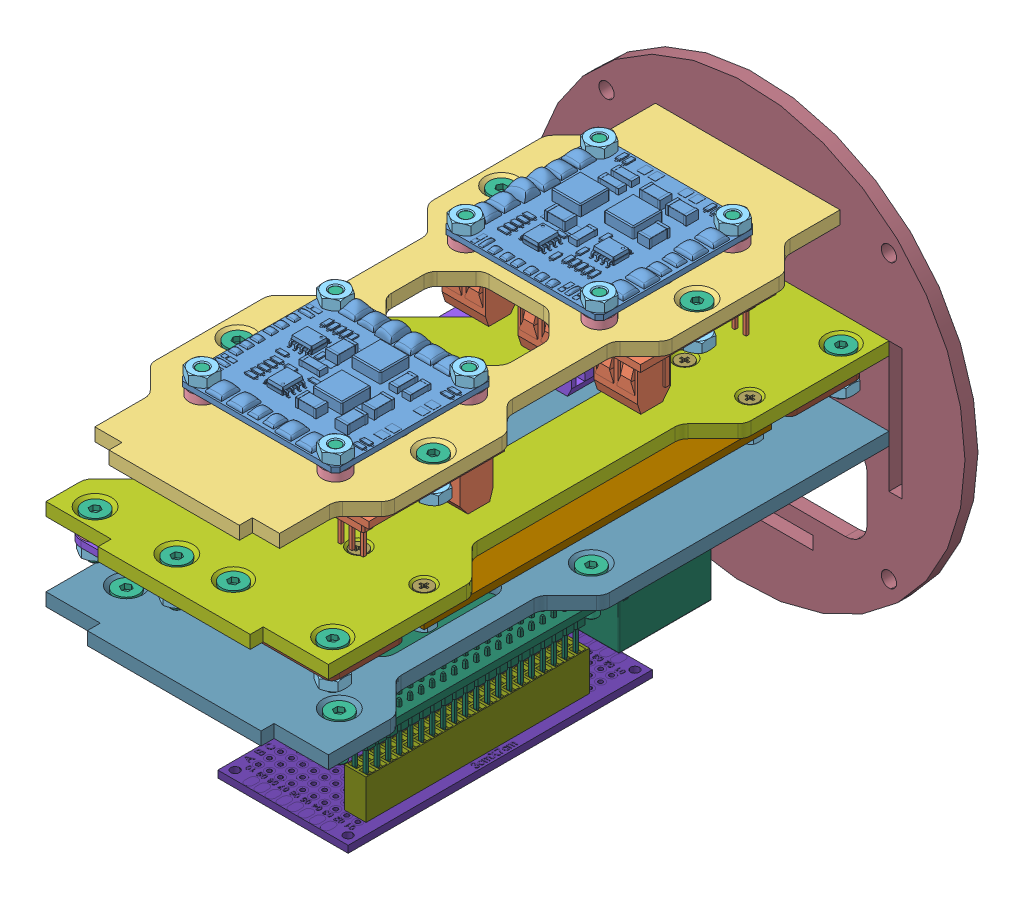
SolidWorks assembly Сборка3, configuration По умолчанию. Lengths in mm.
Overall size (100 100 135).
140 component instances, 17 part files, 9 mates.
Components (placement in the parent):
- ASM-level-power-1: ASM-level-power [По умолчанию] at origin size (55 22.5 135)
  - Matek Power Hub-2: Matek Power Hub [По умолчанию] at (0.0123 -25.5 35.1623) x (0 0 -1) z (1 0 0) size (36.25 3.92 36.25)
  - ACS712.step-1: ACS712.step [По умолчанию] at (17.5 -32.5 34.245) x (0 0 1) z (1 0 0) size (31.19 12.78 13.3)
  - ACS712.step-2: ACS712.step [По умолчанию] at (0 -32.5 34.245) x (0 0 1) z (1 0 0) size (31.19 12.78 13.3)
  - ACS712.step-3: ACS712.step [По умолчанию] at (-17.5 -32.5 34.245) x (0 0 1) z (1 0 0) size (31.19 12.78 13.3)
  - level-0-1: level-0 [По умолчанию] at (0 -30.5 65.5) x (1 0 0) z (0 1 0) size (55 135 3)
  - Matek Power Hub-4: Matek Power Hub [По умолчанию] at (0.0123 -25.5 95.8623) size (36.25 3.92 36.25)
  - ACS712.step-7: ACS712.step [По умолчанию] at (17.5 -32.5 96.755) x (0 0 -1) z (-1 0 0) size (31.19 12.78 13.3)
  - ACS712.step-8: ACS712.step [По умолчанию] at (0 -32.5 96.755) x (0 0 -1) z (-1 0 0) size (31.19 12.78 13.3)
  - ACS712.step-9: ACS712.step [По умолчанию] at (-17.5 -32.5 96.755) x (0 0 -1) z (-1 0 0) size (31.19 12.78 13.3)
  - 3-6-3-1: 3-6-3 [По умолчанию] at (15.35 -27.5 111.2) x (0.999975 0 -0.007062) z (0 1 0) size (6 6 2)
  - 3-6-3-2: 3-6-3 [По умолчанию] at (-15.35 -27.5 111.2) x (0.992437 0 -0.122755) z (0 1 0) size (6 6 2)
  - 3-6-3-3: 3-6-3 [По умолчанию] at (15.35 -27.5 80.5) x (0.931904 0 -0.362706) z (0 1 0) size (6 6 2)
  - 3-6-3-4: 3-6-3 [По умолчанию] at (-15.35 -27.5 80.5) x (1 0 0) z (0 1 0) size (6 6 2)
  - hex nut style 1 gradeab_iso-1: hex nut style 1 gradeab_iso [ISO - 4032 - M3 - D - N] at (15.3745 -21.9 80.5) x (1 0 0) z (0 1 0) size (5.5 6.35 2.4)
  - hex nut style 1 gradeab_iso-2: hex nut style 1 gradeab_iso [ISO - 4032 - M3 - D - N] at (-15.35 -21.9 80.5) x (1 0 0) z (0 1 0) size (5.5 6.35 2.4)
  - hex nut style 1 gradeab_iso-3: hex nut style 1 gradeab_iso [ISO - 4032 - M3 - D - N] at (15.3745 -21.9 111.2245) x (1 0 0) z (0 1 0) size (5.5 6.35 2.4)
  - hex nut style 1 gradeab_iso-4: hex nut style 1 gradeab_iso [ISO - 4032 - M3 - D - N] at (-15.35 -21.9 111.2245) x (1 0 0) z (0 1 0) size (5.5 6.35 2.4)
  - hex nut style 1 gradeab_iso-5: hex nut style 1 gradeab_iso [ISO - 4032 - M3 - D - N] at (15.3745 -21.9 50.5245) x (1 0 0) z (0 1 0) size (5.5 6.35 2.4)
  - hex nut style 1 gradeab_iso-6: hex nut style 1 gradeab_iso [ISO - 4032 - M3 - D - N] at (-15.35 -21.9 50.5245) x (1 0 0) z (0 1 0) size (5.5 6.35 2.4)
  - hex nut style 1 gradeab_iso-7: hex nut style 1 gradeab_iso [ISO - 4032 - M3 - D - N] at (15.3745 -21.9 19.8) x (1 0 0) z (0 1 0) size (5.5 6.35 2.4)
  - hex nut style 1 gradeab_iso-8: hex nut style 1 gradeab_iso [ISO - 4032 - M3 - D - N] at (-15.35 -21.9 19.8) x (1 0 0) z (0 1 0) size (5.5 6.35 2.4)
  - socket countersunk head screw_iso-1: socket countersunk head screw_iso [ISO 10642 - M3 x 8 - 8N] at (15.35 -30.11 111.2) x (0 1 0) z (-0.074206 0 0.997243) size (8 5.54 5.54)
  - socket countersunk head screw_iso-2: socket countersunk head screw_iso [ISO 10642 - M3 x 8 - 8N] at (15.35 -30.11 80.5) x (0 1 0) z (-0.12314 0 0.992389) size (8 5.54 5.54)
  - socket countersunk head screw_iso-3: socket countersunk head screw_iso [ISO 10642 - M3 x 8 - 8N] at (-15.35 -30.11 80.5) x (0 1 0) z (-0.109262 0 0.994013) size (8 5.54 5.54)
  - socket countersunk head screw_iso-4: socket countersunk head screw_iso [ISO 10642 - M3 x 8 - 8N] at (-15.35 -30.11 111.2) x (0 1 0) z (-0.069269 0 0.997598) size (8 5.54 5.54)
  - socket countersunk head screw_iso-5: socket countersunk head screw_iso [ISO 10642 - M3 x 8 - 8N] at (-22.5 -27.89 95.85) x (0 -1 0) z (-0.066693 0 0.997774) size (8 5.54 5.54)
  - socket countersunk head screw_iso-6: socket countersunk head screw_iso [ISO 10642 - M3 x 8 - 8N] at (-12.5 -27.89 95.85) x (0 -1 0) z (-0.00561 0 0.999984) size (8 5.54 5.54)
  - socket countersunk head screw_iso-7: socket countersunk head screw_iso [ISO 10642 - M3 x 8 - 8N] at (-5 -27.89 95.85) x (0 -1 0) z (0.004518 0 0.99999) size (8 5.54 5.54)
  - socket countersunk head screw_iso-8: socket countersunk head screw_iso [ISO 10642 - M3 x 8 - 8N] at (5 -27.89 95.85) x (0 -1 0) z (0.047845 0 0.998855) size (8 5.54 5.54)
  - socket countersunk head screw_iso-9: socket countersunk head screw_iso [ISO 10642 - M3 x 8 - 8N] at (12.5 -27.89 95.85) x (0 -1 0) z (0.031705 0 0.999497) size (8 5.54 5.54)
  - socket countersunk head screw_iso-10: socket countersunk head screw_iso [ISO 10642 - M3 x 8 - 8N] at (22.5 -27.89 95.85) x (0 -1 0) z (0.037692 0 0.999289) size (8 5.54 5.54)
  - hex nut style 1 gradeab_iso-13: hex nut style 1 gradeab_iso [ISO - 4032 - M3 - D - N] at (22.5 -36.48 95.85) x (1 0 0) z (0 -1 0) size (5.5 6.35 2.4)
  - hex nut style 1 gradeab_iso-14: hex nut style 1 gradeab_iso [ISO - 4032 - M3 - D - N] at (12.5 -36.48 95.85) x (1 0 0) z (0 -1 0) size (5.5 6.35 2.4)
  - hex nut style 1 gradeab_iso-15: hex nut style 1 gradeab_iso [ISO - 4032 - M3 - D - N] at (5 -36.48 95.85) x (1 0 0) z (0 -1 0) size (5.5 6.35 2.4)
  - hex nut style 1 gradeab_iso-16: hex nut style 1 gradeab_iso [ISO - 4032 - M3 - D - N] at (-5 -36.48 95.85) x (1 0 0) z (0 -1 0) size (5.5 6.35 2.4)
  - hex nut style 1 gradeab_iso-17: hex nut style 1 gradeab_iso [ISO - 4032 - M3 - D - N] at (-12.5 -36.48 95.85) x (1 0 0) z (0 -1 0) size (5.5 6.35 2.4)
  - hex nut style 1 gradeab_iso-18: hex nut style 1 gradeab_iso [ISO - 4032 - M3 - D - N] at (-22.5 -36.48 95.85) x (1 0 0) z (0 -1 0) size (5.5 6.35 2.4)
  - 3-6-3-5: 3-6-3 [По умолчанию] at (22.5 -32.5 95.85) x (1 0 0) z (0 1 0) size (6 6 2)
  - 3-6-3-6: 3-6-3 [По умолчанию] at (12.5 -32.5 95.85) x (1 0 0) z (0 1 0) size (6 6 2)
  - 3-6-3-7: 3-6-3 [По умолчанию] at (5 -32.5 95.85) x (1 0 0) z (0 1 0) size (6 6 2)
  - 3-6-3-8: 3-6-3 [По умолчанию] at (-5 -32.5 95.85) x (1 0 0) z (0 1 0) size (6 6 2)
  - 3-6-3-9: 3-6-3 [По умолчанию] at (-12.5 -32.5 95.85) x (1 0 0) z (0 1 0) size (6 6 2)
  - 3-6-3-10: 3-6-3 [По умолчанию] at (-22.5 -32.5 95.85) x (1 0 0) z (0 1 0) size (6 6 2)
  - 3-6-3-11: 3-6-3 [По умолчанию] at (-22.5 -30.5 35.15) x (1 0 0) z (0 -1 0) size (6 6 2)
  - hex nut style 1 gradeab_iso-19: hex nut style 1 gradeab_iso [ISO - 4032 - M3 - D - N] at (-22.5 -34.08 35.15) x (1 0 0) z (0 1 0) size (5.5 6.35 2.4)
  - hex nut style 1 gradeab_iso-20: hex nut style 1 gradeab_iso [ISO - 4032 - M3 - D - N] at (-12.5 -34.08 35.15) x (1 0 0) z (0 1 0) size (5.5 6.35 2.4)
  - 3-6-3-12: 3-6-3 [По умолчанию] at (-12.5 -30.5 35.15) x (1 0 0) z (0 -1 0) size (6 6 2)
  - hex nut style 1 gradeab_iso-21: hex nut style 1 gradeab_iso [ISO - 4032 - M3 - D - N] at (-5 -34.08 35.15) x (1 0 0) z (0 1 0) size (5.5 6.35 2.4)
  - hex nut style 1 gradeab_iso-22: hex nut style 1 gradeab_iso [ISO - 4032 - M3 - D - N] at (5 -34.08 35.15) x (1 0 0) z (0 1 0) size (5.5 6.35 2.4)
  - hex nut style 1 gradeab_iso-23: hex nut style 1 gradeab_iso [ISO - 4032 - M3 - D - N] at (12.5 -34.08 35.15) x (1 0 0) z (0 1 0) size (5.5 6.35 2.4)
  - hex nut style 1 gradeab_iso-24: hex nut style 1 gradeab_iso [ISO - 4032 - M3 - D - N] at (22.5 -34.08 35.15) x (1 0 0) z (0 1 0) size (5.5 6.35 2.4)
  - socket countersunk head screw_iso-11: socket countersunk head screw_iso [ISO 10642 - M3 x 8 - 8N] at (22.5 -27.89 35.15) x (0 -1 0) z (-0.037692 0 0.999289) size (8 5.54 5.54)
  - socket countersunk head screw_iso-12: socket countersunk head screw_iso [ISO 10642 - M3 x 8 - 8N] at (12.5 -27.89 35.15) x (0 -1 0) z (-0.031705 0 0.999497) size (8 5.54 5.54)
  - socket countersunk head screw_iso-13: socket countersunk head screw_iso [ISO 10642 - M3 x 8 - 8N] at (5 -27.89 35.15) x (0 -1 0) z (-0.047845 0 0.998855) size (8 5.54 5.54)
  - socket countersunk head screw_iso-14: socket countersunk head screw_iso [ISO 10642 - M3 x 8 - 8N] at (-5 -27.89 35.15) x (0 -1 0) z (-0.004518 0 0.99999) size (8 5.54 5.54)
  - socket countersunk head screw_iso-15: socket countersunk head screw_iso [ISO 10642 - M3 x 8 - 8N] at (-12.5 -27.89 35.15) x (0 -1 0) z (0.00561 0 0.999984) size (8 5.54 5.54)
  - socket countersunk head screw_iso-16: socket countersunk head screw_iso [ISO 10642 - M3 x 8 - 8N] at (-22.5 -27.89 35.15) x (0 -1 0) z (0.066693 0 0.997774) size (8 5.54 5.54)
  - 3-6-3-13: 3-6-3 [По умолчанию] at (-5 -30.5 35.15) x (1 0 0) z (0 -1 0) size (6 6 2)
  - 3-6-3-14: 3-6-3 [По умолчанию] at (5 -30.5 35.15) x (1 0 0) z (0 -1 0) size (6 6 2)
  - 3-6-3-15: 3-6-3 [По умолчанию] at (12.5 -30.5 35.15) x (1 0 0) z (0 -1 0) size (6 6 2)
  - 3-6-3-16: 3-6-3 [По умолчанию] at (22.5 -30.5 35.15) x (1 0 0) z (0 -1 0) size (6 6 2)
  - socket countersunk head screw_iso-17: socket countersunk head screw_iso [ISO 10642 - M3 x 8 - 8N] at (-15.35 -30.11 19.8) x (0 1 0) z (0.069269 0 0.997598) size (8 5.54 5.54)
  - socket countersunk head screw_iso-18: socket countersunk head screw_iso [ISO 10642 - M3 x 8 - 8N] at (15.35 -30.11 19.8) x (0 1 0) z (0.074206 0 0.997243) size (8 5.54 5.54)
  - socket countersunk head screw_iso-19: socket countersunk head screw_iso [ISO 10642 - M3 x 8 - 8N] at (-15.35 -30.11 50.5) x (0 1 0) z (0.109262 0 0.994013) size (8 5.54 5.54)
  - socket countersunk head screw_iso-20: socket countersunk head screw_iso [ISO 10642 - M3 x 8 - 8N] at (15.35 -30.11 50.5) x (0 1 0) z (0.12314 0 0.992389) size (8 5.54 5.54)
  - 3-6-3-17: 3-6-3 [По умолчанию] at (-15.35 -25.5 50.5) x (1 0 0) z (0 -1 0) size (6 6 2)
  - 3-6-3-18: 3-6-3 [По умолчанию] at (-15.35 -25.5 19.8) x (0.992437 0 0.122755) z (0 -1 0) size (6 6 2)
  - 3-6-3-19: 3-6-3 [По умолчанию] at (15.35 -25.5 50.5) x (0.931904 0 0.362706) z (0 -1 0) size (6 6 2)
  - 3-6-3-20: 3-6-3 [По умолчанию] at (15.35 -25.5 19.8) x (0.999975 0 0.007062) z (0 -1 0) size (6 6 2)
- asm-level-pwn-1: asm-level-pwn [По умолчанию] at (0 -48 65.5) x (1 0 0) z (0 -1 0) size (65 135 12.54)
  - level-1-2: level-1 [По умолчанию] at origin size (65 135 3)
  - 3-6-3-33: 3-6-3 [По умолчанию] at (-25.8 -59.9 3) size (6 6 2)
  - 3-6-3-34: 3-6-3 [По умолчанию] at (-7 -59.9 3) size (6 6 2)
  - 3-6-3-35: 3-6-3 [По умолчанию] at (-25.8 -4 3) x (0.841268 -0.540619 0) z (0 0 1) size (6 6 2)
  - 3-6-3-36: 3-6-3 [По умолчанию] at (-7 -4 3) size (6 6 2)
  - 3-6-3-37: 3-6-3 [По умолчанию] at (-25.8 4 3) size (6 6 2)
  - 3-6-3-38: 3-6-3 [По умолчанию] at (-7 4 3) size (6 6 2)
  - 3-6-3-39: 3-6-3 [По умолчанию] at (-25.8 59.9 3) size (6 6 2)
  - 3-6-3-40: 3-6-3 [По умолчанию] at (-7 59.9 3) size (6 6 2)
  - socket countersunk head screw_iso-33: socket countersunk head screw_iso [ISO 10642 - M3 x 10 - 10N] at (-7 -4 0.39) x (0 0 1) z (-0.999892 0.014671 0) size (10 5.54 5.54)
  - socket countersunk head screw_iso-34: socket countersunk head screw_iso [ISO 10642 - M3 x 10 - 10N] at (-7 59.9 0.39) x (0 0 1) z (-0.999933 0.011601 0) size (10 5.54 5.54)
  - socket countersunk head screw_iso-35: socket countersunk head screw_iso [ISO 10642 - M3 x 10 - 10N] at (-25.8 59.9 0.39) x (0 0 1) z (-0.999806 0.019696 0) size (10 5.54 5.54)
  - socket countersunk head screw_iso-36: socket countersunk head screw_iso [ISO 10642 - M3 x 10 - 10N] at (-25.8 4 0.39) x (0 0 1) z (-0.999874 0.015878 0) size (10 5.54 5.54)
  - socket countersunk head screw_iso-37: socket countersunk head screw_iso [ISO 10642 - M3 x 10 - 10N] at (-25.8 -4 0.39) x (0 0 1) z (-0.999899 0.014235 0) size (10 5.54 5.54)
  - socket countersunk head screw_iso-38: socket countersunk head screw_iso [ISO 10642 - M3 x 10 - 10N] at (-7 4 0.39) x (0 0 1) z (-0.999995 0.003285 0) size (10 5.54 5.54)
  - socket countersunk head screw_iso-39: socket countersunk head screw_iso [ISO 10642 - M3 x 10 - 10N] at (-7 -59.9 0.39) x (0 0 1) z (-0.999968 0.008038 0) size (10 5.54 5.54)
  - socket countersunk head screw_iso-40: socket countersunk head screw_iso [ISO 10642 - M3 x 10 - 10N] at (-25.8 -59.9 0.39) x (0 0 1) z (-0.999943 0.010711 0) size (10 5.54 5.54)
  - 12Channel PWM-5: 12Channel PWM [Default] at (-16.4 31.95 5) x (1 0 0) z (0 -1 0) size (25.4 7.55 62.5)
  - 12Channel PWM-6: 12Channel PWM [Default] at (-16.4 -31.95 5) x (1 0 0) z (0 -1 0) size (25.4 7.55 62.5)
  - 20-80-shild-2: 20-80-shild [По умолчанию] at (20 0 5) x (0 -1 0) z (0 0 1) size (80 20 1.6)
  - 2-5-2-1: 2-5-2 [По умолчанию] at (12.5 -37.5 3) size (5 5 2)
  - 2-5-2-2: 2-5-2 [По умолчанию] at (27.5 -37.5 3) x (0.979435 -0.201761 0) z (0 0 1) size (5 5 2)
  - 2-5-2-3: 2-5-2 [По умолчанию] at (12.5 37.5 3) size (5 5 2)
  - 2-5-2-4: 2-5-2 [По умолчанию] at (27.5 37.5 3) size (5 5 2)
  - 16Bit I2C ADC+PGA - ADS1115-3: 16Bit I2C ADC+PGA - ADS1115 [По умолчанию] at (16.07 -52.658 5) x (-1 0 0) z (0 0 1) size (27.94 17.27 2.74)
  - 16Bit I2C ADC+PGA - ADS1115-4: 16Bit I2C ADC+PGA - ADS1115 [По умолчанию] at (16.07 52.658 5) size (27.94 17.27 2.74)
  - 3-6-3-41: 3-6-3 [По умолчанию] at (27.5 58.5 3) x (0.99991 0.013401 0) z (0 0 1) size (6 6 2)
  - 3-6-3-42: 3-6-3 [По умолчанию] at (4.64 58.5 3) size (6 6 2)
  - 3-6-3-43: 3-6-3 [По умолчанию] at (4.64 -58.5 3) x (0.998248 0.059171 0) z (0 0 1) size (6 6 2)
  - 3-6-3-44: 3-6-3 [По умолчанию] at (27.5 -58.5 3) x (0.961366 -0.275274 0) z (0 0 1) size (6 6 2)
  - socket countersunk head screw_iso-41: socket countersunk head screw_iso [ISO 10642 - M3 x 10 - 10N] at (27.5 58.5 0.265) x (0 0 1) z (-0.999931 -0.011786 0) size (10 5.54 5.54)
  - socket countersunk head screw_iso-42: socket countersunk head screw_iso [ISO 10642 - M3 x 10 - 10N] at (4.64 58.5 0.265) x (0 0 1) z (-0.999999 0.001606 0) size (10 5.54 5.54)
  - socket countersunk head screw_iso-43: socket countersunk head screw_iso [ISO 10642 - M3 x 10 - 10N] at (4.64 -58.5 0.265) x (0 0 1) z (-0.999998 -0.001805 0) size (10 5.54 5.54)
  - socket countersunk head screw_iso-44: socket countersunk head screw_iso [ISO 10642 - M3 x 10 - 10N] at (27.5 -58.5 0.265) x (0 0 1) z (-0.999975 -0.007128 0) size (10 5.54 5.54)
  - countersunk flat head cross recess screw_iso-1: countersunk flat head cross recess screw_iso [ISO 7046-1 - M2 x 8 - Z - 8N] at (27.5 -37.5 0.3) x (0 0 1) z (-0.99999 -0.004571 0) size (8 3.8 3.8)
  - countersunk flat head cross recess screw_iso-2: countersunk flat head cross recess screw_iso [ISO 7046-1 - M2 x 8 - Z - 8N] at (12.5 -37.5 0.3) x (0 0 1) z (-0.999692 0.024831 0) size (8 3.8 3.8)
  - countersunk flat head cross recess screw_iso-3: countersunk flat head cross recess screw_iso [ISO 7046-1 - M2 x 8 - Z - 8N] at (27.5 37.5 0.3) x (0 0 1) z (-0.999277 0.038023 0) size (8 3.8 3.8)
  - countersunk flat head cross recess screw_iso-4: countersunk flat head cross recess screw_iso [ISO 7046-1 - M2 x 8 - Z - 8N] at (12.5 37.5 0.3) x (0 0 1) z (-0.999541 0.030296 0) size (8 3.8 3.8)
  - hex nut style 1 gradeab_iso-38: hex nut style 1 gradeab_iso [ISO - 4032 - M3 - D - N] at (4.64 -58.5 9.0002) size (5.5 6.35 2.4)
  - hex nut style 1 gradeab_iso-39: hex nut style 1 gradeab_iso [ISO - 4032 - M3 - D - N] at (27.5 -58.5 9.0002) size (5.5 6.35 2.4)
  - hex nut style 1 gradeab_iso-41: hex nut style 1 gradeab_iso [ISO - 4032 - M3 - D - N] at (-25.8 -59.9 8.91) size (5.5 6.35 2.4)
  - hex nut style 1 gradeab_iso-42: hex nut style 1 gradeab_iso [ISO - 4032 - M3 - D - N] at (-7 4 8.91) size (5.5 6.35 2.4)
  - hex nut style 1 gradeab_iso-43: hex nut style 1 gradeab_iso [ISO - 4032 - M3 - D - N] at (-7 -4 8.9) size (5.5 6.35 2.4)
  - hex nut style 1 gradeab_iso-44: hex nut style 1 gradeab_iso [ISO - 4032 - M3 - D - N] at (-25.8 4 8.91) size (5.5 6.35 2.4)
  - hex nut style 1 gradeab_iso-45: hex nut style 1 gradeab_iso [ISO - 4032 - M3 - D - N] at (-25.8 -4 8.91) size (5.5 6.35 2.4)
  - hex nut style 1 gradeab_iso-46: hex nut style 1 gradeab_iso [ISO - 4032 - M3 - D - N] at (-25.8 59.9 8.91) size (5.5 6.35 2.4)
  - hex nut style 1 gradeab_iso-47: hex nut style 1 gradeab_iso [ISO - 4032 - M3 - D - N] at (-7 59.9 8.9) size (5.5 6.35 2.4)
  - hex nut style 1 gradeab_iso-48: hex nut style 1 gradeab_iso [ISO - 4032 - M3 - D - N] at (4.64 58.5 9.0002) size (5.5 6.35 2.4)
  - hex nut style 1 gradeab_iso-50: hex nut style 1 gradeab_iso [ISO - 4032 - M3 - D - N] at (-7 -59.9 8.91) size (5.5 6.35 2.4)
  - hex nut style 1 gradeab_iso-51: hex nut style 1 gradeab_iso [ISO - 4032 - M3 - D - N] at (27.5 58.5 9.0002) size (5.5 6.35 2.4)
  - hex nut style 1 gradeab_iso-52: hex nut style 1 gradeab_iso [ISO - 4032 - M2 - D - N] at (12.5 -37.5 8.2) size (4 4.62 1.6)
  - hex nut style 1 gradeab_iso-53: hex nut style 1 gradeab_iso [ISO - 4032 - M2 - D - N] at (27.5 -37.5 8.2) size (4 4.62 1.6)
  - hex nut style 1 gradeab_iso-54: hex nut style 1 gradeab_iso [ISO - 4032 - M2 - D - N] at (12.5 37.5 8.2) size (4 4.62 1.6)
  - hex nut style 1 gradeab_iso-55: hex nut style 1 gradeab_iso [ISO - 4032 - M2 - D - N] at (27.5 37.5 8.2) size (4 4.62 1.6)
- baze-100mm-1: baze-100mm [По умолчанию] at (0 -63 -2) x (-1 0 0) z (0 0 1) size (100 100 3)
- ASM-level-raspberry-pi-1: ASM-level-raspberry-pi [По умолчанию] at (0 -66 65.5) x (-1 0 0) z (0 -1 0) size (65 135 24.74)
  - level-2-1: level-2 [По умолчанию] at origin size (65 135 3)
  - Raspberry Pi 4 Model B-1: Raspberry Pi 4 Model B [По умолчанию] at (0 -15 5.79) x (0 1 0) z (1 0 0) size (88.99 19.91 58.4)
  - 3-6-3-1: 3-6-3 [По умолчанию] at (-24.5 -54 3) size (6 6 2)
  - 3-6-3-2: 3-6-3 [По умолчанию] at (-24.5 4 3) size (6 6 2)
  - 3-6-3-3: 3-6-3 [По умолчанию] at (24.5 4 3) size (6 6 2)
  - 3-6-3-4: 3-6-3 [По умолчанию] at (24.5 -54 3) x (0.98212 -0.188257 0) z (0 0 1) size (6 6 2)
  - socket countersunk head screw_iso-1: socket countersunk head screw_iso [ISO 10642 - M3 x 10 - 10N] at (24.5 -54 0.39) x (0 0 1) z (-0.999977 -0.006797 0) size (10 5.54 5.54)
  - socket countersunk head screw_iso-2: socket countersunk head screw_iso [ISO 10642 - M3 x 10 - 10N] at (24.5 4 0.39) x (0 0 1) z (-0.999917 -0.012873 0) size (10 5.54 5.54)
  - socket countersunk head screw_iso-3: socket countersunk head screw_iso [ISO 10642 - M3 x 10 - 10N] at (-24.5 4 0.39) x (0 0 1) z (-0.999928 -0.012001 0) size (10 5.54 5.54)
  - socket countersunk head screw_iso-4: socket countersunk head screw_iso [ISO 10642 - M3 x 10 - 10N] at (-24.5 -54 0.39) x (0 0 1) z (-1 -0.000767 0) size (10 5.54 5.54)
  - ASM-shild-raspberry-1: ASM-shild-raspberry [По умолчанию] at (-22.18 0.88 25.14) x (1 0 0) z (0 1 0) size (30 10.65 70)
    - 40 pin connector header smt v3.step-1: 40 pin connector header smt v3.step [По умолчанию] at origin size (5.18 10.05 51.4)
    - Breadboard 30 х 70 mm.step-1: Breadboard 30 х 70 mm.step [По умолчанию] at (7.5097 0.4 -23.0097) size (30 1.65 70)
Mates (geometry in assembly coordinates):
- Совпадение1: coincident anti-aligned: plane of ASM-level-power-1/level-0-1 through (0 -27.5 65.5) normal (0 1 0); plane of baze-100mm-1 through (15 -27.5 -7) normal (0 -1 0)
- Совпадение2: coincident anti-aligned: plane of ASM-level-power-1/level-0-1 through (-15 -27.5 65.5) normal (-1 0 0); plane of baze-100mm-1 through (-15 -30.5 -7) normal (1 0 0)
- Совпадение3: coincident anti-aligned: plane of ASM-level-power-1/level-0-1 through (0 -27.5 1) normal (0 0 -1); plane of baze-100mm-1 through (0 -63 1) normal (0 0 1)
- Совпадение4: coincident anti-aligned: plane of asm-level-pwn-1/level-1-2 through (17.5 -51 65.5) normal (1 0 0); plane of baze-100mm-1 through (17.5 -51 -7) normal (-1 0 0)
- Совпадение5: coincident anti-aligned: plane of asm-level-pwn-1/level-1-2 through (0 -48 65.5) normal (0 1 0); plane of baze-100mm-1 through (17.5 -48 -7) normal (0 -1 0)
- Совпадение6: coincident anti-aligned: plane of asm-level-pwn-1/level-1-2 through (0 -51 1) normal (0 0 -1); plane of baze-100mm-1 through (0 -63 1) normal (0 0 1)
- Совпадение71: coincident anti-aligned: plane of baze-100mm-1 through (20 -69 -7) normal (0 1 0); plane of ASM-level-raspberry-pi-1/level-2-1 through (0 -69 65.5) normal (0 -1 0)
- Совпадение8: coincident anti-aligned: plane of baze-100mm-1 through (0 -63 1) normal (0 0 1); plane of ASM-level-raspberry-pi-1/level-2-1 through (0 -69 1) normal (0 0 -1)
- Совпадение9: coincident anti-aligned: plane of baze-100mm-1 through (-20 -69 -7) normal (1 0 0); plane of ASM-level-raspberry-pi-1/level-2-1 through (-20 -69 65.5) normal (-1 0 0)
